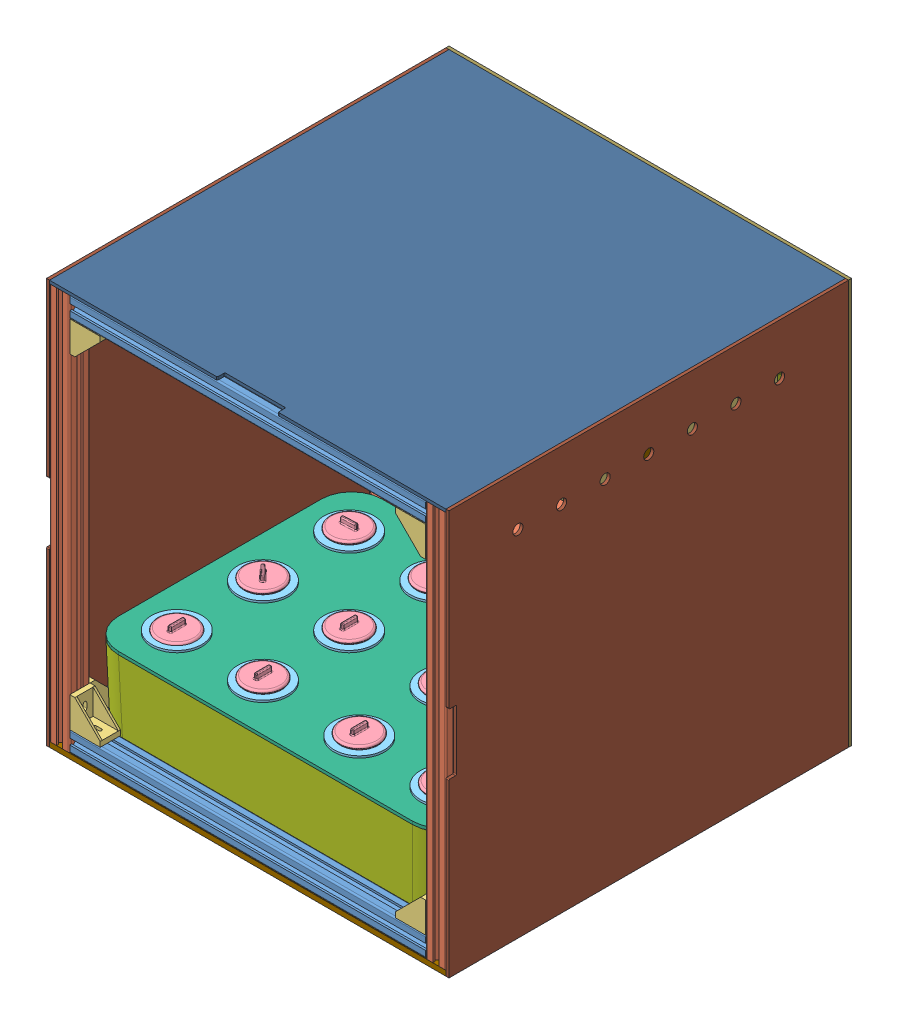
SolidWorks assembly skeleton_v2, configuration 預設. Lengths in mm. (continued)
Mates (geometry in assembly coordinates): (continued)
- 重合/共線/共點271: coincident aligned: plane of Fixedcomponent_middle-3 through (369.3054 -262.2141 340) normal (0 0 -1); plane of Fixedcomponent_middle-5 through (369.3054 -122.2141 340) normal (0 0 -1)
- 重合/共線/共點272: coincident aligned: plane of Fixedcomponent_middle-3 through (369.3054 -262.2141 340) normal (0 0 -1); plane of Fixedcomponent_middle-7 through (369.3054 -402.2141 340) normal (0 0 -1)
- 重合/共線/共點273: coincident aligned: plane of Fixedcomponent_middle-3 through (377.0554 -262.2141 340) normal (1 0 0); plane of Fixedcomponent_middle-7 through (377.0554 -402.2141 340) normal (1 0 0)
- 重合/共線/共點274: coincident anti-aligned: plane of Fixedcomponent_middle-3 through (341.8036 -262.2141 342.3593) normal (0 -1 0); plane of Fixedcomponent_middle-7 through (341.8036 -262.2141 342.3593) normal (0 1 0)
- 重合/共線/共點275: coincident anti-aligned: plane of Fixedcomponent_middle-9 through (21.3071 -262.2141 342.3593) normal (0 -1 0); plane of Fixedcomponent_middle-10 through (21.3071 -262.2141 342.3593) normal (0 1 0)
- 重合/共線/共點276: coincident aligned: plane of Fixedcomponent_middle-8 through (-13.9446 -402.2141 340) normal (-1 0 0); plane of Fixedcomponent_middle-9 through (-13.9446 -122.2141 340) normal (-1 0 0)
- 重合/共線/共點277: coincident aligned: plane of Fixedcomponent_middle-8 through (-13.9446 -402.2141 340) normal (-1 0 0); plane of Fixedcomponent_middle-10 through (-13.9446 -262.2141 340) normal (-1 0 0)
- 重合/共線/共點278: coincident aligned: plane of Fixedcomponent_middle-8 through (-6.1946 -402.2141 340) normal (0 0 -1); plane of Fixedcomponent_middle-10 through (-6.1946 -262.2141 340) normal (0 0 -1)
- 重合/共線/共點279: coincident aligned: plane of Fixedcomponent_middle-11 through (-13.9446 157.7859 340) normal (-1 0 0); plane of Fixedcomponent_middle-12 through (-13.9446 17.7859 340) normal (-1 0 0)
- 重合/共線/共點280: coincident aligned: plane of Fixedcomponent_middle-11 through (-6.1946 157.7859 340) normal (0 0 -1); plane of Fixedcomponent_middle-12 through (-6.1946 17.7859 340) normal (0 0 -1)
- 重合/共線/共點281: coincident anti-aligned: plane of Fixedcomponent_middle-9 through (21.3071 -122.2141 342.3593) normal (0 1 0); plane of Fixedcomponent_middle-12 through (21.3071 -122.2141 342.3593) normal (0 -1 0)
- 重合/共線/共點282: coincident aligned: plane of Fixedcomponent_middle-9 through (-6.1946 -122.2141 340) normal (0 0 -1); plane of Fixedcomponent_middle-12 through (-6.1946 17.7859 340) normal (0 0 -1)
- 重合/共線/共點283: coincident anti-aligned: plane of Fixedcomponent_middle-11 through (21.3071 17.7859 342.3593) normal (0 -1 0); plane of Fixedcomponent_middle-12 through (21.3071 17.7859 342.3593) normal (0 1 0)
- 重合/共線/共點284: coincident aligned: plane of Fixedcomponent_middle-9 through (-13.9446 -122.2141 344) normal (0 0 1); plane of Fixedcomponent_middle-10 through (-13.9446 -262.2141 344) normal (0 0 1)
- 重合/共線/共點285: coincident anti-aligned: plane of Fixedcomponent_middle-8 through (21.3071 -402.2141 342.3593) normal (0 1 0); plane of Fixedcomponent_middle-10 through (21.3071 -402.2141 342.3593) normal (0 -1 0)
- 重合/共線/共點286: coincident aligned: plane of Fixedcomponent_middle-10 through (-13.9446 -262.2141 340) normal (-1 0 0); plane of Fixedcomponent_middle-12 through (-13.9446 17.7859 340) normal (-1 0 0)
- 重合/共線/共點287: coincident aligned: plane of Fixedcomponent-13 through (-67.368 142.6997 267.7916) normal (0 0 1); plane of Fixedcomponent-14 through (-67.368 127.6997 267.7916) normal (0 0 1)
- 重合/共線/共點288: coincident anti-aligned: plane of Fixedcomponent-13 through (-32.1163 127.6997 266.1509) normal (0 -1 0); plane of Fixedcomponent-14 through (-32.1163 127.6997 266.1509) normal (0 1 0)
- 重合/共線/共點289: coincident aligned: plane of Fixedcomponent-14 through (-67.368 127.6997 263.7916) normal (-1 0 0); plane of Fixedcomponent-17 through (-67.368 112.6997 263.7916) normal (-1 0 0)
- 重合/共線/共點290: coincident anti-aligned: plane of Fixedcomponent-13 through (-32.1163 142.6997 266.1509) normal (0 1 0); plane of Fixedcomponent-16 through (-32.1163 142.6997 266.1509) normal (0 -1 0)
- 重合/共線/共點291: coincident aligned: plane of Fixedcomponent_middle-15 through (369.3054 -1242.2141 340) normal (0 0 -1); plane of Fixedcomponent-16 through (-59.618 157.6997 263.7916) normal (0 0 -1)
- 重合/共線/共點292: coincident aligned: plane of Fixedcomponent_middle-15 through (377.0554 -1242.2141 340) normal (1 0 0); plane of Fixedcomponent-16 through (-67.368 157.6997 263.7916) normal (-1 0 0)
- 重合/共線/共點293: coincident anti-aligned: plane of Fixedcomponent_middle-15 through (341.8036 -1102.2141 342.3593) normal (0 1 0); plane of Fixedcomponent-16 through (-32.1163 157.6997 266.1509) normal (0 1 0)
- 重合/共線/共點294: coincident aligned: plane of Fixedcomponent-13 through (-67.368 142.6997 263.7916) normal (-1 0 0); plane of Fixedcomponent-17 through (-67.368 112.6997 263.7916) normal (-1 0 0)
- 重合/共線/共點295: coincident anti-aligned: plane of Fixedcomponent-14 through (-32.1163 112.6997 266.1509) normal (0 -1 0); plane of Fixedcomponent-17 through (-32.1163 112.6997 266.1509) normal (0 1 0)
- 重合/共線/共點296: coincident aligned: plane of Fixedcomponent-13 through (-59.618 142.6997 263.7916) normal (0 0 -1); plane of Fixedcomponent-16 through (-59.618 157.6997 263.7916) normal (0 0 -1)
- 重合/共線/共點297: coincident aligned: plane of Fixedcomponent-14 through (-67.368 127.6997 263.7916) normal (-1 0 0); plane of Fixedcomponent-16 through (-67.368 157.6997 263.7916) normal (-1 0 0)
- 重合/共線/共點298: coincident aligned: plane of Fixedcomponent-14 through (-59.618 127.6997 263.7916) normal (0 0 -1); plane of Fixedcomponent-17 through (-59.618 112.6997 263.7916) normal (0 0 -1)
- 重合/共線/共點299: coincident aligned: plane of Fixedcomponent_middle-2 through (-13.9446 297.7859 340) normal (-1 0 0); plane of Fixedcomponent_middle-12 through (-13.9446 17.7859 340) normal (-1 0 0)
- 重合/共線/共點300: coincident anti-aligned: plane of Fixedcomponent_middle-2 through (21.3071 157.7859 342.3593) normal (0 -1 0); plane of Fixedcomponent_middle-11 through (21.3071 157.7859 342.3593) normal (0 1 0)
- 重合/共線/共點301: coincident aligned: plane of Fixedcomponent_middle-2 through (-6.1946 297.7859 340) normal (0 0 -1); plane of Fixedcomponent_middle-11 through (-6.1946 157.7859 340) normal (0 0 -1)
- 重合/共線/共點302: coincident aligned: plane of Fixedcomponent_middle-19 through (-13.9446 -542.2141 340) normal (-1 0 0); plane of Fixedcomponent_middle-20 through (-13.9446 -682.2141 340) normal (-1 0 0)
- 重合/共線/共點303: coincident aligned: plane of Fixedcomponent_middle-18 through (-13.9446 -962.2141 344) normal (0 0 1); plane of Fixedcomponent_middle-22 through (-13.9446 -822.2141 344) normal (0 0 1)
- 重合/共線/共點304: coincident anti-aligned: plane of Fixedcomponent_middle-18 through (21.3071 -962.2141 342.3593) normal (0 1 0); plane of Fixedcomponent_middle-22 through (21.3071 -962.2141 342.3593) normal (0 -1 0)
- 重合/共線/共點305: coincident aligned: plane of Fixedcomponent_middle-19 through (-6.1946 -542.2141 340) normal (0 0 -1); plane of Fixedcomponent_middle-20 through (-6.1946 -682.2141 340) normal (0 0 -1)
- 重合/共線/共點306: coincident anti-aligned: plane of Fixedcomponent_middle-20 through (21.3071 -822.2141 342.3593) normal (0 -1 0); plane of Fixedcomponent_middle-22 through (21.3071 -822.2141 342.3593) normal (0 1 0)
- 重合/共線/共點307: coincident anti-aligned: plane of Fixedcomponent_middle-19 through (21.3071 -682.2141 342.3593) normal (0 -1 0); plane of Fixedcomponent_middle-20 through (21.3071 -682.2141 342.3593) normal (0 1 0)
- 重合/共線/共點308: coincident aligned: plane of Fixedcomponent_middle-18 through (-13.9446 -962.2141 340) normal (-1 0 0); plane of Fixedcomponent_middle-21 through (-13.9446 -1102.2141 340) normal (-1 0 0)
- 重合/共線/共點309: coincident anti-aligned: plane of Fixedcomponent_middle-18 through (21.3071 -1102.2141 342.3593) normal (0 -1 0); plane of Fixedcomponent_middle-21 through (21.3071 -1102.2141 342.3593) normal (0 1 0)
- 重合/共線/共點310: coincident aligned: plane of Fixedcomponent_middle-18 through (-13.9446 -962.2141 340) normal (-1 0 0); plane of Fixedcomponent_middle-20 through (-13.9446 -682.2141 340) normal (-1 0 0)
- 重合/共線/共點311: coincident aligned: plane of Fixedcomponent_middle-18 through (-6.1946 -962.2141 340) normal (0 0 -1); plane of Fixedcomponent_middle-21 through (-6.1946 -1102.2141 340) normal (0 0 -1)
- 重合/共線/共點312: coincident aligned: plane of Fixedcomponent_middle-20 through (-6.1946 -682.2141 340) normal (0 0 -1); plane of Fixedcomponent_middle-22 through (-6.1946 -822.2141 340) normal (0 0 -1)
- 重合/共線/共點313: coincident aligned: plane of Fixedcomponent_middle-21 through (-13.9446 -1102.2141 340) normal (-1 0 0); plane of Fixedcomponent_middle-22 through (-13.9446 -822.2141 340) normal (-1 0 0)
- 重合/共線/共點314: coincident aligned: plane of Fixedcomponent_middle-24 through (297.0586 379.1322 340) normal (0 1 0); plane of Fixedcomponent_middle-25 through (157.0586 379.1322 340) normal (0 1 0)
- 重合/共線/共點315: coincident aligned: plane of Fixedcomponent_middle-23 through (-122.9414 379.1322 344) normal (0 0 1); plane of Fixedcomponent_middle-27 through (17.0586 379.1322 344) normal (0 0 1)
- 重合/共線/共點316: coincident anti-aligned: plane of Fixedcomponent_middle-23 through (-122.9414 343.8805 342.3593) normal (1 0 0); plane of Fixedcomponent_middle-27 through (-122.9414 343.8805 342.3593) normal (-1 0 0)
- 重合/共線/共點317: coincident aligned: plane of Fixedcomponent_middle-24 through (297.0586 371.3822 340) normal (0 0 -1); plane of Fixedcomponent_middle-25 through (157.0586 371.3822 340) normal (0 0 -1)
- 重合/共線/共點318: coincident anti-aligned: plane of Fixedcomponent_middle-25 through (17.0586 343.8805 342.3593) normal (-1 0 0); plane of Fixedcomponent_middle-27 through (17.0586 343.8805 342.3593) normal (1 0 0)
- 重合/共線/共點319: coincident anti-aligned: plane of Fixedcomponent_middle-24 through (157.0586 343.8805 342.3593) normal (-1 0 0); plane of Fixedcomponent_middle-25 through (157.0586 343.8805 342.3593) normal (1 0 0)
- 重合/共線/共點320: coincident aligned: plane of Fixedcomponent_middle-23 through (-122.9414 379.1322 340) normal (0 1 0); plane of Fixedcomponent_middle-26 through (-262.9414 379.1322 340) normal (0 1 0)
- 重合/共線/共點321: coincident anti-aligned: plane of Fixedcomponent_middle-23 through (-262.9414 343.8805 342.3593) normal (-1 0 0); plane of Fixedcomponent_middle-26 through (-262.9414 343.8805 342.3593) normal (1 0 0)
- 重合/共線/共點322: coincident aligned: plane of Fixedcomponent_middle-23 through (-122.9414 379.1322 340) normal (0 1 0); plane of Fixedcomponent_middle-25 through (157.0586 379.1322 340) normal (0 1 0)
- 重合/共線/共點323: coincident aligned: plane of Fixedcomponent_middle-23 through (-122.9414 371.3822 340) normal (0 0 -1); plane of Fixedcomponent_middle-26 through (-262.9414 371.3822 340) normal (0 0 -1)
- 重合/共線/共點324: coincident aligned: plane of Fixedcomponent_middle-25 through (157.0586 371.3822 340) normal (0 0 -1); plane of Fixedcomponent_middle-27 through (17.0586 371.3822 340) normal (0 0 -1)
- 重合/共線/共點325: coincident aligned: plane of Fixedcomponent_middle-26 through (-262.9414 379.1322 340) normal (0 1 0); plane of Fixedcomponent_middle-27 through (17.0586 379.1322 340) normal (0 1 0)
- 重合/共線/共點326: coincident aligned: plane of Fixedcomponent_middle-29 through (766.0522 379.1322 340) normal (0 1 0); plane of Fixedcomponent_middle-30 through (626.0522 379.1322 340) normal (0 1 0)
- 重合/共線/共點327: coincident aligned: plane of Fixedcomponent_middle-28 through (346.0522 379.1322 344) normal (0 0 1); plane of Fixedcomponent_middle-32 through (486.0522 379.1322 344) normal (0 0 1)
- 重合/共線/共點328: coincident anti-aligned: plane of Fixedcomponent_middle-28 through (346.0522 343.8805 342.3593) normal (1 0 0); plane of Fixedcomponent_middle-32 through (346.0522 343.8805 342.3593) normal (-1 0 0)
- 重合/共線/共點329: coincident aligned: plane of Fixedcomponent_middle-29 through (766.0522 371.3822 340) normal (0 0 -1); plane of Fixedcomponent_middle-30 through (626.0522 371.3822 340) normal (0 0 -1)
- 重合/共線/共點330: coincident anti-aligned: plane of Fixedcomponent_middle-30 through (486.0522 343.8805 342.3593) normal (-1 0 0); plane of Fixedcomponent_middle-32 through (486.0522 343.8805 342.3593) normal (1 0 0)
- 重合/共線/共點331: coincident anti-aligned: plane of Fixedcomponent_middle-29 through (626.0522 343.8805 342.3593) normal (-1 0 0); plane of Fixedcomponent_middle-30 through (626.0522 343.8805 342.3593) normal (1 0 0)
- 重合/共線/共點332: coincident aligned: plane of Fixedcomponent_middle-28 through (346.0522 379.1322 340) normal (0 1 0); plane of Fixedcomponent_middle-31 through (206.2372 379.1322 340) normal (0 1 0)
- 重合/共線/共點333: coincident anti-aligned: plane of Fixedcomponent_middle-28 through (206.0522 343.8805 342.3593) normal (-1 0 0); plane of Fixedcomponent_middle-31 through (206.2372 343.8805 342.3593) normal (1 0 0)
- 重合/共線/共點334: coincident aligned: plane of Fixedcomponent_middle-28 through (346.0522 379.1322 340) normal (0 1 0); plane of Fixedcomponent_middle-30 through (626.0522 379.1322 340) normal (0 1 0)
- 重合/共線/共點335: coincident aligned: plane of Fixedcomponent_middle-28 through (346.0522 371.3822 340) normal (0 0 -1); plane of Fixedcomponent_middle-31 through (206.2372 371.3822 340) normal (0 0 -1)
- 重合/共線/共點336: coincident aligned: plane of Fixedcomponent_middle-30 through (626.0522 371.3822 340) normal (0 0 -1); plane of Fixedcomponent_middle-32 through (486.0522 371.3822 340) normal (0 0 -1)
- 重合/共線/共點337: coincident aligned: plane of Fixedcomponent_middle-31 through (206.2372 379.1322 340) normal (0 1 0); plane of Fixedcomponent_middle-32 through (486.0522 379.1322 340) normal (0 1 0)
- 重合/共線/共點338: coincident aligned: plane of Fixedcomponent_middle-8 through (-13.9446 -402.2141 340) normal (-1 0 0); plane of Fixedcomponent_middle-19 through (-13.9446 -542.2141 340) normal (-1 0 0)
- 重合/共線/共點339: coincident aligned: plane of Fixedcomponent_middle-8 through (-6.1946 -402.2141 340) normal (0 0 -1); plane of Fixedcomponent_middle-20 through (-6.1946 -682.2141 340) normal (0 0 -1)
- 重合/共線/共點340: coincident anti-aligned: plane of Fixedcomponent_middle-8 through (21.3071 -542.2141 342.3593) normal (0 -1 0); plane of Fixedcomponent_middle-19 through (21.3071 -542.2141 342.3593) normal (0 1 0)
- 重合/共線/共點341: coincident anti-aligned: plane of Fixedcomponent_middle-34 through (1046.0522 343.8805 342.3593) normal (-1 0 0); plane of Fixedcomponent_middle-35 through (1046.0522 343.8805 342.3593) normal (1 0 0)
- 重合/共線/共點342: coincident aligned: plane of Fixedcomponent_middle-33 through (906.0522 379.1322 340) normal (0 1 0); plane of Fixedcomponent_middle-34 through (1186.0522 379.1322 340) normal (0 1 0)
- 重合/共線/共點343: coincident aligned: plane of Fixedcomponent_middle-33 through (906.0522 379.1322 340) normal (0 1 0); plane of Fixedcomponent_middle-35 through (1046.0522 379.1322 340) normal (0 1 0)
- 重合/共線/共點344: coincident aligned: plane of Fixedcomponent_middle-33 through (906.0522 371.3822 340) normal (0 0 -1); plane of Fixedcomponent_middle-35 through (1046.0522 371.3822 340) normal (0 0 -1)
- 重合/共線/共點345: coincident aligned: plane of Fixedcomponent_middle-36 through (1466.0522 379.1322 340) normal (0 1 0); plane of Fixedcomponent_middle-37 through (1326.0522 379.1322 340) normal (0 1 0)
- 重合/共線/共點346: coincident aligned: plane of Fixedcomponent_middle-36 through (1466.0522 371.3822 340) normal (0 0 -1); plane of Fixedcomponent_middle-37 through (1326.0522 371.3822 340) normal (0 0 -1)
- 重合/共線/共點347: coincident anti-aligned: plane of Fixedcomponent_middle-34 through (1186.0522 343.8805 342.3593) normal (1 0 0); plane of Fixedcomponent_middle-37 through (1186.0522 343.8805 342.3593) normal (-1 0 0)
- 重合/共線/共點348: coincident aligned: plane of Fixedcomponent_middle-34 through (1186.0522 371.3822 340) normal (0 0 -1); plane of Fixedcomponent_middle-37 through (1326.0522 371.3822 340) normal (0 0 -1)
- 重合/共線/共點349: coincident anti-aligned: plane of Fixedcomponent_middle-36 through (1326.0522 343.8805 342.3593) normal (-1 0 0); plane of Fixedcomponent_middle-37 through (1326.0522 343.8805 342.3593) normal (1 0 0)
- 重合/共線/共點350: coincident aligned: plane of Fixedcomponent_middle-34 through (1186.0522 379.1322 344) normal (0 0 1); plane of Fixedcomponent_middle-35 through (1046.0522 379.1322 344) normal (0 0 1)
- 重合/共線/共點351: coincident anti-aligned: plane of Fixedcomponent_middle-33 through (906.0522 343.8805 342.3593) normal (1 0 0); plane of Fixedcomponent_middle-35 through (906.0522 343.8805 342.3593) normal (-1 0 0)
- 重合/共線/共點352: coincident aligned: plane of Fixedcomponent_middle-35 through (1046.0522 379.1322 340) normal (0 1 0); plane of Fixedcomponent_middle-37 through (1326.0522 379.1322 340) normal (0 1 0)
- 重合/共線/共點353: coincident anti-aligned: plane of Fixedcomponent_middle-29 through (766.0522 343.8805 342.3593) normal (1 0 0); plane of Fixedcomponent_middle-33 through (766.0522 343.8805 342.3593) normal (-1 0 0)
- 重合/共線/共點354: coincident aligned: plane of Fixedcomponent_middle-30 through (626.0522 379.1322 340) normal (0 1 0); plane of Fixedcomponent_middle-33 through (906.0522 379.1322 340) normal (0 1 0)
- 重合/共線/共點355: coincident aligned: plane of Fixedcomponent_middle-29 through (766.0522 379.1322 344) normal (0 0 1); plane of Fixedcomponent_middle-33 through (906.0522 379.1322 344) normal (0 0 1)
- 重合/共線/共點357: coincident aligned: plane of FixedcomponentWithtri-2 through (66.2372 371.3822 340) normal (0 0 -1); plane of Fixedcomponent_middle-31 through (206.2372 371.3822 340) normal (0 0 -1)
- 重合/共線/共點358: coincident aligned: plane of FixedcomponentWithtri-2 through (66.2372 379.1322 340) normal (0 1 0); plane of Fixedcomponent_middle-31 through (206.2372 379.1322 340) normal (0 1 0)
- 重合/共線/共點359: coincident anti-aligned: plane of plate_side-2 through (377.0554 182.6322 514) normal (-1 0 0); plane of FixedcomponentWithtriright-1 through (377.0554 328.936 344) normal (1 0 0)
- 重合/共線/共點360: coincident anti-aligned: plane of plate_top-1 through (181.5554 379.1322 514) normal (0 -1 0); plane of FixedcomponentWithtriright-1 through (296.8586 379.1322 340) normal (0 1 0)
- 重合/共線/共點361: coincident anti-aligned: line of Fixedcomponent_middle-36 through (1466.0522 327.5188 320) axis (0 1 0); plane of FixedcomponentWithtriright-1 through (301.8586 343.8805 320) normal (0 0 -1)
- 重合/共線/共點362: coincident anti-aligned: plane of Fixedcomponent_middle-39 through (341.8036 -682.2141 342.3593) normal (0 1 0); plane of Fixedcomponent_middle-40 through (341.8036 -682.2141 342.3593) normal (0 -1 0)
- 重合/共線/共點363: coincident aligned: plane of Fixedcomponent_middle-38 through (377.0554 -542.2141 340) normal (1 0 0); plane of Fixedcomponent_middle-39 through (377.0554 -822.2141 340) normal (1 0 0)
- 重合/共線/共點364: coincident aligned: plane of Fixedcomponent_middle-38 through (377.0554 -542.2141 340) normal (1 0 0); plane of Fixedcomponent_middle-40 through (377.0554 -682.2141 340) normal (1 0 0)
- 重合/共線/共點365: coincident aligned: plane of Fixedcomponent_middle-38 through (369.3054 -542.2141 340) normal (0 0 -1); plane of Fixedcomponent_middle-40 through (369.3054 -682.2141 340) normal (0 0 -1)
- 重合/共線/共點366: coincident aligned: plane of Fixedcomponent_middle-41 through (377.0554 -1102.2141 340) normal (1 0 0); plane of Fixedcomponent_middle-42 through (377.0554 -962.2141 340) normal (1 0 0)
- 重合/共線/共點367: coincident aligned: plane of Fixedcomponent_middle-41 through (369.3054 -1102.2141 340) normal (0 0 -1); plane of Fixedcomponent_middle-42 through (369.3054 -962.2141 340) normal (0 0 -1)
- 重合/共線/共點368: coincident anti-aligned: plane of Fixedcomponent_middle-39 through (341.8036 -822.2141 342.3593) normal (0 -1 0); plane of Fixedcomponent_middle-42 through (341.8036 -822.2141 342.3593) normal (0 1 0)
- 重合/共線/共點369: coincident aligned: plane of Fixedcomponent_middle-39 through (369.3054 -822.2141 340) normal (0 0 -1); plane of Fixedcomponent_middle-42 through (369.3054 -962.2141 340) normal (0 0 -1)
- 重合/共線/共點370: coincident anti-aligned: plane of Fixedcomponent_middle-41 through (341.8036 -962.2141 342.3593) normal (0 1 0); plane of Fixedcomponent_middle-42 through (341.8036 -962.2141 342.3593) normal (0 -1 0)
- 重合/共線/共點371: coincident aligned: plane of Fixedcomponent_middle-39 through (377.0554 -822.2141 344) normal (0 0 1); plane of Fixedcomponent_middle-40 through (377.0554 -682.2141 344) normal (0 0 1)
- 重合/共線/共點372: coincident anti-aligned: plane of Fixedcomponent_middle-38 through (341.8036 -542.2141 342.3593) normal (0 -1 0); plane of Fixedcomponent_middle-40 through (341.8036 -542.2141 342.3593) normal (0 1 0)
- 重合/共線/共點373: coincident aligned: plane of Fixedcomponent_middle-40 through (377.0554 -682.2141 340) normal (1 0 0); plane of Fixedcomponent_middle-42 through (377.0554 -962.2141 340) normal (1 0 0)
- 重合/共線/共點386: coincident anti-aligned: plane of Fixedcomponent_middle-7 through (341.8036 -402.2141 342.3593) normal (0 -1 0); plane of Fixedcomponent_middle-38 through (341.8036 -402.2141 342.3593) normal (0 1 0)
- 重合/共線/共點387: coincident aligned: plane of Fixedcomponent_middle-7 through (377.0554 -402.2141 344) normal (0 0 1); plane of Fixedcomponent_middle-38 through (377.0554 -542.2141 344) normal (0 0 1)
- 重合/共線/共點388: coincident aligned: plane of Fixedcomponent_middle-7 through (377.0554 -402.2141 340) normal (1 0 0); plane of Fixedcomponent_middle-38 through (377.0554 -542.2141 340) normal (1 0 0)
- 重合/共線/共點389: coincident anti-aligned: plane of Fixedcomponent_middle-24 through (297.0586 343.8805 342.3593) normal (1 0 0); plane of FixedcomponentWithtriright-1 through (296.8586 343.8805 342.3593) normal (-1 0 0)
- 重合/共線/共點390: coincident anti-aligned: plane of plate_back-1 through (181.5554 183.6322 320) normal (0 0 1); plane of Fixedcomponent_middle-26 through (-262.9414 331.3488 320) normal (0 0 -1)
- 重合/共線/共點391: coincident aligned: plane of Fixedcomponent_middle-26 through (-262.9414 379.1322 340) normal (0 1 0); plane of Fixedcomponent_middle-36 through (1466.0522 379.1322 340) normal (0 1 0)
- 重合/共線/共點392: coincident anti-aligned: plane of plate_side-2 through (377.0554 182.6322 514) normal (-1 0 0); plane of Fixedcomponent_middle-41 through (377.0554 -1102.2141 340) normal (1 0 0)
- 重合/共線/共點393: coincident anti-aligned: plane of plate_back-1 through (181.5554 183.6322 320) normal (0 0 1); plane of Fixedcomponent_middle-42 through (329.272 -962.2141 320) normal (0 0 -1)
- 重合/共線/共點394: coincident anti-aligned: plane of Fixedcomponent-4 through (341.8036 297.7859 342.3593) normal (0 1 0); plane of FixedcomponentWithtriright-1 through (353.1054 297.7859 320) normal (0 -1 0)
- 重合/共線/共點395: coincident anti-aligned: plane of plate_side-2 through (377.0554 182.6322 514) normal (-1 0 0); plane of Fixedcomponent_middle-15 through (377.0554 -1242.2141 340) normal (1 0 0)
- 重合/共線/共點396: coincident anti-aligned: plane of plate_back-1 through (181.5554 183.6322 320) normal (0 0 1); plane of Fixedcomponent_middle-15 through (329.272 -1242.2141 320) normal (0 0 -1)
- 重合/共線/共點397: coincident anti-aligned: plane of Fixedcomponent_middle-15 through (341.8036 -1102.2141 342.3593) normal (0 1 0); plane of Fixedcomponent_middle-41 through (341.8036 -1102.2141 342.3593) normal (0 -1 0)
- 重合/共線/共點398: coincident aligned: plane of Fixedcomponent_middle-15 through (341.8036 -1242.2141 342.3593) normal (0 -1 0); plane of Assem1-1/raspberry pi test-1 through (206.2372 144.5864 322) normal (0 -1 0)
- 重合/共線/共點400: coincident: line of Fixedcomponent_middle-37 through (1326.0522 379.1322 344) axis (0 -1 0); plane of Assem1-1/raspberry pi test-1 through (206.2372 144.5864 322) normal (1 0 0)
- 重合/共線/共點401: coincident anti-aligned: plane of plate_back-1 through (181.5554 183.6322 320) normal (0 0 1); plane of Assem1-1/raspberry pi test-1 through (185.8137 159.8307 320) normal (0 0 -1)
- 重合/共線/共點402: coincident: line of plate_side-2 through (380.0554 -16.8678 317) axis (0 1 0); plane of plate_door-2 through (181.5554 182.6322 317) normal (0 0 1)
- 重合/共線/共點403: coincident anti-aligned: plane of controlbox_right-3 through (106.0554 78.1322 433) normal (-1 0 0); plane of controlbox_left-1 through (106.0554 63.1322 340) normal (1 0 0)
- 重合/共線/共點404: coincident anti-aligned: plane of plate_bottom-1 through (181.5554 -11.8678 514) normal (0 1 0); plane of 1219 ControlBox version-1/1219 ground-1 through (357.0554 -11.8678 419) normal (0 -1 0)
- 重合/共線/共點410: coincident anti-aligned: plane of stick_2020_340-8 through (357.0554 8.1322 340) normal (0 0 1); plane of 1219 ControlBox version-1/1219 roof-1 through (320.6845 26.144 340) normal (0 0 -1)
- 重合/共線/共點413: coincident anti-aligned: plane of stick_2020_340-6 through (357.0554 8.1322 340) normal (-1 0 0); plane of 1219 ControlBox version-1/1219 ground-1 through (357.0554 76.1322 419) normal (1 0 0)
- 重合/共線/共點415: coincident anti-aligned: plane of stick_2020_340-1 through (6.0554 8.1322 691) normal (1 0 0); plane of controlbox_left-1 through (6.0554 71.1322 433) normal (-1 0 0)
- 重合/共線/共點416: coincident anti-aligned: plane of stick_2020_340-8 through (357.0554 8.1322 340) normal (0 0 1); plane of controlbox_left-1 through (116.0554 71.1322 340) normal (0 0 -1)
- 重合/共線/共點417: coincident anti-aligned: plane of controlbox_left-1 through (116.0554 71.1322 386.5) normal (0 1 0); plane of controlbox_lid-1 through (116.1055 71.1322 386.7449) normal (0 -1 0)
- 相切2: tangent aligned: cylinder of controlbox_lid-1 through (196.1556 66.1322 370.4898) axis (0 1 0) radius 25.5; cylinder of controlbox_left-1 through (196.0554 71.1322 370) axis (0 -1 0) radius 26
- 同軸心20: concentric aligned: cylinder of controlbox_left-1 through (36.0554 71.1322 403) axis (0 1 0) radius 26; cylinder of controlbox_lid-1 through (36.0554 66.1322 403) axis (0 1 0) radius 25.5
- 重合/共線/共點418: coincident anti-aligned: plane of lid_v2-1 through (181.0554 81.1322 562.9859) normal (0 1 0); plane of ring-15 through (228.5554 81.1322 477.9859) normal (0 -1 0)
- 重合/共線/共點419: coincident anti-aligned: plane of lid_v2-1 through (181.0554 81.1322 562.9859) normal (0 1 0); plane of ring-11 through (313.5554 81.1322 477.9859) normal (0 -1 0)
- 重合/共線/共點420: coincident anti-aligned: plane of lid_v2-1 through (181.0554 81.1322 562.9859) normal (0 1 0); plane of ring-14 through (228.5554 81.1322 562.9859) normal (0 -1 0)
- 重合/共線/共點421: coincident anti-aligned: plane of lid_v2-1 through (181.0554 81.1322 562.9859) normal (0 1 0); plane of ring-13 through (228.5554 81.1322 647.9859) normal (0 -1 0)
- 重合/共線/共點422: coincident anti-aligned: plane of lid_v2-1 through (181.0554 81.1322 562.9859) normal (0 1 0); plane of ring-12 through (313.5554 81.1322 562.9859) normal (0 -1 0)
- 同軸心21: concentric aligned: cylinder of lid_v2-1 through (228.5554 78.1312 477.9859) axis (0 1 0) radius 22; cylinder of ring-15 through (228.5554 77.8822 477.9859) axis (0 1 0) radius 15.5
- 同軸心22: concentric aligned: cylinder of lid_v2-1 through (228.5554 78.1312 562.9859) axis (0 1 0) radius 22; cylinder of ring-14 through (228.5554 77.8822 562.9859) axis (0 1 0) radius 15.5
- 同軸心23: concentric aligned: cylinder of lid_v2-1 through (228.5554 78.1312 647.9859) axis (0 1 0) radius 22; cylinder of ring-13 through (228.5554 77.8822 647.9859) axis (0 1 0) radius 15.5
- 同軸心24: concentric aligned: cylinder of lid_v2-1 through (313.5554 78.1312 477.9859) axis (0 1 0) radius 22; cylinder of ring-11 through (313.5554 77.8822 477.9859) axis (0 1 0) radius 15.5
- 同軸心25: concentric aligned: cylinder of lid_v2-1 through (313.5554 78.1312 562.9859) axis (0 1 0) radius 22; cylinder of ring-12 through (313.5554 77.8822 562.9859) axis (0 1 0) radius 15.5
- 重合/共線/共點423: coincident anti-aligned: plane of lid_v2-1 through (181.0554 81.1322 562.9859) normal (0 1 0); plane of ring-16 through (313.5554 81.1322 647.9859) normal (0 -1 0)
- 同軸心26: concentric aligned: cylinder of lid_v2-1 through (313.5554 78.1312 647.9859) axis (0 1 0) radius 22; cylinder of ring-16 through (313.5554 77.8822 647.9859) axis (0 1 0) radius 15.5
- 同軸心27: concentric aligned: cylinder of ring-1 through (48.5554 77.8822 477.9859) axis (0 1 0) radius 15.5; cylinder of small fixed lid with EC sensor and temperture-1 through (48.5554 79.1322 477.9859) axis (0 1 0) radius 14.75
- 重合/共線/共點424: coincident anti-aligned: plane of ring-1 through (48.5554 83.1322 477.9859) normal (0 1 0); plane of small fixed lid with EC sensor and temperture-4 through (19.7064 83.1322 641.3464) normal (0 -1 0)
- 重合/共線/共點425: coincident anti-aligned: plane of ring-9 through (133.5554 83.1322 562.9859) normal (0 1 0); plane of small fixed lid with EC sensor and temperture-2 through (104.7064 83.1322 556.3464) normal (0 -1 0)
- 重合/共線/共點426: coincident anti-aligned: plane of ring-3 through (48.5554 83.1322 647.9859) normal (0 1 0); plane of small fixed lid with EC sensor and temperture-1 through (25.7411 83.1322 496.85) normal (0 -1 0)
- 重合/共線/共點427: coincident anti-aligned: plane of ring-14 through (228.5554 83.1322 562.9859) normal (0 1 0); plane of small fixed lid with EC sensor and temperture-5 through (199.7064 83.1322 556.3464) normal (0 -1 0)
- 重合/共線/共點428: coincident anti-aligned: plane of ring-11 through (313.5554 83.1322 477.9859) normal (0 1 0); plane of small fixed lid with EC sensor and temperture-3 through (329.9868 83.1034 508.6938) normal (0 -1 0)
- 重合/共線/共點429: coincident anti-aligned: plane of ring-16 through (313.5554 83.1322 647.9859) normal (0 1 0); plane of small fixed lid with EC sensor and temperture-6 through (284.7064 83.1322 556.3464) normal (0 -1 0)
- 同軸心28: concentric aligned: cylinder of ring-3 through (48.5554 77.8822 647.9859) axis (0 1 0) radius 15.5; cylinder of small fixed lid with EC sensor and temperture-4 through (48.5554 79.1322 647.9859) axis (0 1 0) radius 14.75
- 同軸心29: concentric aligned: cylinder of ring-9 through (133.5554 77.8822 562.9859) axis (0 1 0) radius 15.5; cylinder of small fixed lid with EC sensor and temperture-2 through (133.5554 79.1322 562.9859) axis (0 1 0) radius 14.75
- 同軸心30: concentric aligned: cylinder of ring-14 through (228.5554 77.8822 562.9859) axis (0 1 0) radius 15.5; cylinder of small fixed lid with EC sensor and temperture-5 through (228.5554 79.1322 562.9859) axis (0 1 0) radius 14.75
- 重合/共線/共點430: coincident anti-aligned: plane of plate_back-1 through (181.5554 183.6322 320) normal (0 0 1); plane of Assem1-1/raspberry pi test-1 through (185.8137 159.8307 320) normal (0 0 -1)
- 重合/共線/共點431: coincident aligned: plane of Fixedcomponent_middle-2 through (21.3071 157.7859 342.3593) normal (0 -1 0); plane of Assem1-1/raspberry pi test-1 through (206.2372 144.5864 322) normal (0 -1 0)
- 重合/共線/共點432: coincident anti-aligned: plane of FixedcomponentWithtri-2 through (10.0054 297.7683 320) normal (0 -1 0); plane of Fixedcomponent_left-43 through (21.3071 297.7683 342.3593) normal (0 1 0)
- 重合/共線/共點433: coincident aligned: plane of FixedcomponentWithtri-2 through (61.2372 343.8805 340) normal (0 0 -1); plane of Fixedcomponent_left-43 through (-6.1946 297.7683 340) normal (0 0 -1)
- 重合/共線/共點434: coincident aligned: plane of FixedcomponentWithtri-2 through (-13.9446 328.921 344) normal (-1 0 0); plane of Fixedcomponent_left-43 through (-13.9446 297.7683 340) normal (-1 0 0)
- 重合/共線/共點435: coincident aligned: plane of FixedcomponentWithtriright-1 through (377.0554 328.936 344) normal (1 0 0); plane of Fixedcomponent_right-43 through (377.0554 97.7859 340) normal (1 0 0)
- 重合/共線/共點436: coincident anti-aligned: plane of FixedcomponentWithtriright-1 through (353.1054 297.7859 320) normal (0 -1 0); plane of Fixedcomponent_right-43 through (341.8036 297.7859 342.3593) normal (0 1 0)
- 重合/共線/共點438: coincident anti-aligned: plane of plate_back-1 through (181.5554 183.6322 320) normal (0 0 1); plane of Fixedcomponent_right-43 through (329.472 97.7859 320) normal (0 0 -1)
- 重合/共線/共點439: coincident aligned: plane of Fixedcomponent_middle-31 through (206.2372 343.8805 342.3593) normal (1 0 0); plane of Assem1-1/raspberry pi test-1 through (206.2372 144.5864 322) normal (1 0 0)
- 重合/共線/共點440: coincident anti-aligned: plane of Fixedcomponent_right-43 through (341.8036 297.7859 342.3593) normal (0 1 0); plane of FixedcomponentWithtriright-2 through (353.1054 297.7859 320) normal (0 -1 0)
- 重合/共線/共點441: coincident aligned: plane of Fixedcomponent_right-43 through (377.0554 97.7859 340) normal (1 0 0); plane of FixedcomponentWithtriright-2 through (377.0554 328.9386 344) normal (1 0 0)
- 重合/共線/共點442: coincident anti-aligned: plane of stick_2020_380-4 through (357.0554 -11.8678 340) normal (0 0 1); plane of FixedcomponentWithtriright-2 through (301.8736 343.8981 340) normal (0 0 -1)
- 重合/共線/共點444: coincident aligned: plane of stick_2020_380-4 through (377.0554 -11.8678 320) normal (1 0 0); plane of FixedcomponentWithtriright-2 through (377.0554 328.9386 344) normal (1 0 0)
- 重合/共線/共點445: coincident anti-aligned: plane of FixedcomponentWithtri-2 through (66.2372 343.8805 342.3593) normal (1 0 0); plane of Fixedcomponent_middle-31 through (66.2372 343.8805 342.3593) normal (-1 0 0)
- 重合/共線/共點446: coincident: plane of stick_2020_380-2 through (-13.9446 -11.8678 340) normal (0 0 1); plane of 90 Degree Cast Corner for 2020 Extrusion (Ooznest).step-1 through (-5.4446 349.1322 340) normal (0 0 -1)
- 重合/共線/共點447: coincident: plane of stick_2020_340-3 through (-13.9446 359.1322 691) normal (0 -1 0); plane of 90 Degree Cast Corner for 2020 Extrusion (Ooznest).step-1 through (3.0554 359.1322 340) normal (0 1 0)
- 重合/共線/共點448: coincident aligned: plane of stick_2020_380-2 through (-13.9446 -11.8678 320) normal (-1 0 0); plane of 90 Degree Cast Corner for 2020 Extrusion (Ooznest).step-1 through (-13.9446 359.1322 340) normal (-1 0 0)
- 重合/共線/共點449: coincident anti-aligned: plane of stick_2020_380-2 through (-13.9446 -11.8678 340) normal (0 0 1); plane of Aluminium extrusion connector-1 through (6.0554 359.1322 340) normal (0 0 -1)
- 重合/共線/共點450: coincident anti-aligned: plane of stick_2020_340-3 through (-13.9446 359.1322 691) normal (0 -1 0); plane of Aluminium extrusion connector-1 through (6.0554 359.1322 370) normal (0 1 0)
- 重合/共線/共點451: coincident aligned: plane of stick_2020_340-3 through (-13.9446 379.1322 691) normal (-1 0 0); plane of Aluminium extrusion connector-1 through (-13.9446 359.1322 370) normal (-1 0 0)
- 重合/共線/共點452: coincident anti-aligned: plane of stick_2020_380-4 through (357.0554 -11.8678 340) normal (0 0 1); plane of Aluminium extrusion connector-5 through (377.0554 359.1322 340) normal (0 0 -1)
- 重合/共線/共點453: coincident anti-aligned: plane of stick_2020_340-7 through (377.0554 359.1322 340) normal (0 -1 0); plane of Aluminium extrusion connector-5 through (377.0554 359.1322 370) normal (0 1 0)
- 重合/共線/共點454: coincident aligned: plane of stick_2020_380-4 through (377.0554 -11.8678 320) normal (1 0 0); plane of Aluminium extrusion connector-5 through (377.0554 359.1322 370) normal (1 0 0)
- 重合/共線/共點455: coincident anti-aligned: plane of stick_2020_340-7 through (377.0554 359.1322 340) normal (0 -1 0); plane of Aluminium extrusion connector-4 through (357.0554 359.1322 661) normal (0 1 0)
- 重合/共線/共點456: coincident anti-aligned: plane of stick_2020_380-3 through (357.0554 -11.8678 691) normal (0 0 -1); plane of Aluminium extrusion connector-4 through (357.0554 359.1322 691) normal (0 0 1)
- 重合/共線/共點457: coincident aligned: plane of stick_2020_340-7 through (377.0554 379.1322 340) normal (1 0 0); plane of Aluminium extrusion connector-4 through (377.0554 359.1322 661) normal (1 0 0)
- 重合/共線/共點458: coincident anti-aligned: plane of stick_2020_340-4 through (6.0554 359.1322 691) normal (0 -1 0); plane of Aluminium extrusion connector-2 through (357.0554 359.1322 691) normal (0 1 0)
- 重合/共線/共點459: coincident anti-aligned: plane of stick_2020_380-3 through (357.0554 -11.8678 691) normal (-1 0 0); plane of Aluminium extrusion connector-2 through (357.0554 329.1322 691) normal (1 0 0)
- 重合/共線/共點460: coincident aligned: plane of stick_2020_340-4 through (6.0554 379.1322 711) normal (0 0 1); plane of Aluminium extrusion connector-2 through (357.0554 329.1322 711) normal (0 0 1)
- 重合/共線/共點461: coincident anti-aligned: plane of stick_2020_340-4 through (6.0554 379.1322 691) normal (0 0 -1); plane of Aluminium extrusion connector-3 through (327.0554 359.1322 691) normal (0 0 1)
- 重合/共線/共點462: coincident anti-aligned: plane of stick_2020_340-7 through (357.0554 379.1322 340) normal (-1 0 0); plane of Aluminium extrusion connector-3 through (357.0554 359.1322 691) normal (1 0 0)
- 重合/共線/共點463: coincident aligned: plane of stick_2020_340-7 through (377.0554 359.1322 340) normal (0 -1 0); plane of Aluminium extrusion connector-3 through (327.0554 359.1322 691) normal (0 -1 0)
- 重合/共線/共點464: coincident anti-aligned: plane of stick_2020_380-4 through (357.0554 -11.8678 320) normal (-1 0 0); plane of Aluminium extrusion connector-9 through (357.0554 359.1322 340) normal (1 0 0)
- 重合/共線/共點465: coincident anti-aligned: plane of stick_2020_340-5 through (6.0554 359.1322 320) normal (0 -1 0); plane of Aluminium extrusion connector-9 through (327.0554 359.1322 340) normal (0 1 0)
- 重合/共線/共點466: coincident aligned: plane of stick_2020_380-4 through (357.0554 -11.8678 320) normal (0 0 -1); plane of Aluminium extrusion connector-9 through (327.0554 359.1322 320) normal (0 0 -1)
- 重合/共線/共點467: coincident anti-aligned: plane of stick_2020_380-4 through (357.0554 -11.8678 340) normal (0 0 1); plane of Aluminium extrusion connector-7 through (357.0554 8.1322 340) normal (0 0 -1)
- 重合/共線/共點468: coincident anti-aligned: plane of stick_2020_340-6 through (377.0554 8.1322 340) normal (0 1 0); plane of Aluminium extrusion connector-7 through (357.0554 8.1322 370) normal (0 -1 0)
- 重合/共線/共點469: coincident aligned: plane of stick_2020_380-4 through (377.0554 -11.8678 320) normal (1 0 0); plane of Aluminium extrusion connector-7 through (377.0554 8.1322 370) normal (1 0 0)
- 重合/共線/共點470: coincident anti-aligned: plane of stick_2020_340-4 through (6.0554 379.1322 691) normal (0 0 -1); plane of Aluminium extrusion connector-8 through (6.0554 359.1322 691) normal (0 0 1)
- 重合/共線/共點471: coincident anti-aligned: plane of stick_2020_340-3 through (6.0554 379.1322 691) normal (1 0 0); plane of Aluminium extrusion connector-8 through (6.0554 359.1322 661) normal (-1 0 0)
- 重合/共線/共點472: coincident aligned: plane of stick_2020_340-3 through (-13.9446 379.1322 691) normal (0 1 0); plane of Aluminium extrusion connector-8 through (6.0554 379.1322 661) normal (0 1 0)
- 重合/共線/共點473: coincident anti-aligned: plane of Aluminium extrusion connector-6 through (6.0554 329.1322 691) normal (0 0 1); plane of stick_2020_380-1 through (-13.9446 -11.8678 691) normal (0 0 -1)
- 重合/共線/共點474: coincident anti-aligned: plane of stick_2020_340-3 through (-13.9446 359.1322 691) normal (0 -1 0); plane of Aluminium extrusion connector-6 through (6.0554 359.1322 691) normal (0 1 0)
- 重合/共線/共點476: coincident aligned: plane of stick_2020_340-3 through (-13.9446 379.1322 691) normal (-1 0 0); plane of Aluminium extrusion connector-6 through (-13.9446 329.1322 691) normal (-1 0 0)
- 重合/共線/共點477: coincident aligned: plane of stick_2020_380-1 through (-13.9446 -11.8678 711) normal (0 0 1); plane of Aluminium extrusion connector-18 through (6.0554 38.1322 711) normal (0 0 1)
- 重合/共線/共點478: coincident anti-aligned: plane of stick_2020_340-2 through (6.0554 8.1322 691) normal (0 1 0); plane of Aluminium extrusion connector-18 through (6.0554 8.1322 691) normal (0 -1 0)
- 重合/共線/共點479: coincident anti-aligned: plane of stick_2020_380-1 through (6.0554 -11.8678 691) normal (1 0 0); plane of Aluminium extrusion connector-18 through (6.0554 38.1322 691) normal (-1 0 0)
- 重合/共線/共點480: coincident anti-aligned: plane of stick_2020_340-1 through (-13.9446 8.1322 691) normal (0 1 0); plane of Aluminium extrusion connector-19 through (-13.9446 8.1322 691) normal (0 -1 0)
- 重合/共線/共點481: coincident anti-aligned: plane of stick_2020_380-1 through (-13.9446 -11.8678 691) normal (0 0 -1); plane of Aluminium extrusion connector-19 through (-13.9446 38.1322 691) normal (0 0 1)
- 重合/共線/共點482: coincident aligned: plane of stick_2020_380-1 through (-13.9446 -11.8678 691) normal (-1 0 0); plane of Aluminium extrusion connector-19 through (-13.9446 38.1322 691) normal (-1 0 0)
- 重合/共線/共點483: coincident anti-aligned: plane of stick_2020_380-2 through (6.0554 -11.8678 320) normal (1 0 0); plane of Aluminium extrusion connector-17 through (6.0554 38.1322 320) normal (-1 0 0)
- 重合/共線/共點484: coincident aligned: plane of stick_2020_380-2 through (-13.9446 -11.8678 340) normal (0 0 1); plane of Aluminium extrusion connector-17 through (6.0554 38.1322 340) normal (0 0 1)
- 重合/共線/共點485: coincident anti-aligned: plane of stick_2020_340-8 through (357.0554 8.1322 320) normal (0 1 0); plane of Aluminium extrusion connector-17 through (6.0554 8.1322 320) normal (0 -1 0)
- 重合/共線/共點486: coincident anti-aligned: plane of stick_2020_380-4 through (357.0554 -11.8678 320) normal (-1 0 0); plane of Aluminium extrusion connector-16 through (357.0554 38.1322 340) normal (1 0 0)
- 重合/共線/共點487: coincident anti-aligned: plane of stick_2020_340-8 through (357.0554 8.1322 320) normal (0 1 0); plane of Aluminium extrusion connector-16 through (357.0554 8.1322 340) normal (0 -1 0)
- 重合/共線/共點488: coincident aligned: plane of stick_2020_380-4 through (357.0554 -11.8678 320) normal (0 0 -1); plane of Aluminium extrusion connector-16 through (357.0554 38.1322 320) normal (0 0 -1)
- 重合/共線/共點489: coincident anti-aligned: plane of stick_2020_380-2 through (-13.9446 -11.8678 340) normal (0 0 1); plane of Aluminium extrusion connector-13 through (6.0554 38.1322 340) normal (0 0 -1)
- 重合/共線/共點490: coincident anti-aligned: plane of stick_2020_340-1 through (-13.9446 8.1322 691) normal (0 1 0); plane of Aluminium extrusion connector-13 through (6.0554 8.1322 340) normal (0 -1 0)
- 重合/共線/共點491: coincident aligned: plane of stick_2020_380-2 through (-13.9446 -11.8678 320) normal (-1 0 0); plane of Aluminium extrusion connector-13 through (-13.9446 38.1322 340) normal (-1 0 0)
- 重合/共線/共點493: coincident anti-aligned: plane of stick_2020_340-5 through (6.0554 359.1322 320) normal (0 -1 0); plane of Aluminium extrusion connector-15 through (6.0554 359.1322 340) normal (0 1 0)
- 重合/共線/共點494: coincident aligned: plane of stick_2020_340-5 through (6.0554 379.1322 320) normal (0 0 -1); plane of Aluminium extrusion connector-15 through (6.0554 329.1322 320) normal (0 0 -1)
- 重合/共線/共點495: coincident anti-aligned: plane of stick_2020_380-2 through (6.0554 -11.8678 320) normal (1 0 0); plane of Aluminium extrusion connector-15 through (6.0554 329.1322 340) normal (-1 0 0)
- 重合/共線/共點496: coincident anti-aligned: plane of stick_2020_380-1 through (6.0554 -11.8678 691) normal (1 0 0); plane of Aluminium extrusion connector-20 through (6.0554 359.1322 691) normal (-1 0 0)
- 重合/共線/共點497: coincident anti-aligned: plane of stick_2020_340-4 through (6.0554 359.1322 691) normal (0 -1 0); plane of Aluminium extrusion connector-20 through (36.0554 359.1322 691) normal (0 1 0)
- 重合/共線/共點498: coincident aligned: plane of stick_2020_380-1 through (-13.9446 -11.8678 711) normal (0 0 1); plane of Aluminium extrusion connector-20 through (36.0554 359.1322 711) normal (0 0 1)
- 重合/共線/共點499: coincident anti-aligned: plane of stick_2020_340-6 through (377.0554 8.1322 340) normal (0 1 0); plane of Aluminium extrusion connector-14 through (357.0554 8.1322 691) normal (0 -1 0)
- 重合/共線/共點500: coincident anti-aligned: plane of stick_2020_380-3 through (357.0554 -11.8678 691) normal (0 0 -1); plane of Aluminium extrusion connector-14 through (357.0554 38.1322 691) normal (0 0 1)
- 重合/共線/共點501: coincident aligned: plane of stick_2020_380-3 through (377.0554 -11.8678 691) normal (1 0 0); plane of Aluminium extrusion connector-14 through (377.0554 38.1322 691) normal (1 0 0)
- 重合/共線/共點502: coincident anti-aligned: plane of stick_2020_340-2 through (6.0554 8.1322 691) normal (0 1 0); plane of Aluminium extrusion connector-12 through (357.0554 8.1322 711) normal (0 -1 0)
- 重合/共線/共點503: coincident anti-aligned: plane of stick_2020_380-3 through (357.0554 -11.8678 691) normal (-1 0 0); plane of Aluminium extrusion connector-12 through (357.0554 38.1322 711) normal (1 0 0)
- 重合/共線/共點504: coincident aligned: plane of stick_2020_380-3 through (357.0554 -11.8678 711) normal (0 0 1); plane of Aluminium extrusion connector-12 through (357.0554 38.1322 711) normal (0 0 1)
- 重合/共線/共點505: coincident anti-aligned: plane of lid_v2-1 through (181.0554 81.1322 562.9859) normal (0 1 0); plane of ring-17 through (48.5554 81.1322 477.9859) normal (0 -1 0)
- 同軸心33: concentric aligned: cylinder of lid_v2-1 through (48.5554 78.1312 477.9859) axis (0 1 0) radius 22; cylinder of ring-17 through (48.5554 77.8822 477.9859) axis (0 1 0) radius 15.5
- 同軸心34: concentric aligned: cylinder of ring-2 through (48.5554 77.8822 562.9859) axis (0 1 0) radius 15.5; cylinder of small lid-1 through (48.5554 73.1322 562.9859) axis (0 1 0) radius 14.5
- 重合/共線/共點506: coincident anti-aligned: plane of ring-2 through (48.5554 83.1322 562.9859) normal (0 1 0); plane of small lid-1 through (48.5554 83.1322 562.9859) normal (0 -1 0)
- 同軸心35: concentric aligned: cylinder of small fixed lid with EC sensor and temperture-6 through (313.5554 79.1322 562.9859) axis (0 1 0) radius 14.75; cylinder of ring-12 through (313.5554 77.8822 562.9859) axis (0 1 0) radius 15.5
- 重合/共線/共點507: coincident anti-aligned: plane of lid_v2-1 through (181.0554 81.1322 562.9859) normal (0 1 0); plane of small lid-2 through (48.5554 81.1322 647.9859) normal (0 -1 0)
- 同軸心36: concentric aligned: cylinder of ring-3 through (48.5554 77.8822 647.9859) axis (0 1 0) radius 15.5; cylinder of small lid-2 through (48.5554 71.1322 647.9859) axis (0 1 0) radius 14.5
- 重合/共線/共點508: coincident anti-aligned: plane of ring-10 through (133.5554 83.1322 647.9859) normal (0 1 0); plane of small lid-11 through (133.5554 83.1322 647.9859) normal (0 -1 0)
- 同軸心37: concentric aligned: cylinder of ring-10 through (133.5554 77.8822 647.9859) axis (0 1 0) radius 15.5; cylinder of small lid-11 through (133.5554 73.1322 647.9859) axis (0 1 0) radius 14.5
- 重合/共線/共點509: coincident anti-aligned: plane of ring-13 through (228.5554 83.1322 647.9859) normal (0 1 0); plane of small lid-5 through (228.5554 83.1322 647.9859) normal (0 -1 0)
- 同軸心38: concentric aligned: cylinder of ring-13 through (228.5554 77.8822 647.9859) axis (0 1 0) radius 15.5; cylinder of small lid-5 through (228.5554 73.1322 647.9859) axis (0 1 0) radius 14.5
- 重合/共線/共點510: coincident anti-aligned: plane of ring-9 through (133.5554 83.1322 562.9859) normal (0 1 0); plane of small lid-7 through (133.5554 83.1322 562.9859) normal (0 -1 0)
- 同軸心39: concentric aligned: cylinder of ring-9 through (133.5554 77.8822 562.9859) axis (0 1 0) radius 15.5; cylinder of small lid-7 through (133.5554 73.1322 562.9859) axis (0 1 0) radius 14.5
- 同軸心40: concentric aligned: cylinder of ring-14 through (228.5554 77.8822 562.9859) axis (0 1 0) radius 15.5; cylinder of small lid-8 through (228.5554 73.1322 562.9859) axis (0 1 0) radius 14.5
- 重合/共線/共點511: coincident anti-aligned: plane of ring-14 through (228.5554 83.1322 562.9859) normal (0 1 0); plane of small lid-8 through (228.5554 83.1322 562.9859) normal (0 -1 0)
- 同軸心41: concentric aligned: cylinder of ring-17 through (48.5554 77.8822 477.9859) axis (0 1 0) radius 15.5; cylinder of small lid-6 through (48.5554 73.1322 477.9859) axis (0 1 0) radius 14.5
- 重合/共線/共點512: coincident anti-aligned: plane of ring-17 through (48.5554 83.1322 477.9859) normal (0 1 0); plane of small lid-6 through (48.5554 83.1322 477.9859) normal (0 -1 0)
- 重合/共線/共點513: coincident anti-aligned: plane of ring-16 through (313.5554 83.1322 647.9859) normal (0 1 0); plane of small lid-9 through (313.5554 83.1322 647.9859) normal (0 -1 0)
- 同軸心42: concentric aligned: cylinder of ring-16 through (313.5554 77.8822 647.9859) axis (0 1 0) radius 15.5; cylinder of small lid-9 through (313.5554 73.1322 647.9859) axis (0 1 0) radius 14.5
- 同軸心43: concentric aligned: circle of ring-6; cylinder of small lid-10 through (133.5554 73.1322 477.9859) axis (0 1 0) radius 14.5
- 重合/共線/共點514: coincident anti-aligned: plane of ring-6 through (133.5554 83.1322 477.9859) normal (0 1 0); plane of small lid-10 through (133.5554 83.1322 477.9859) normal (0 -1 0)
- 同軸心44: concentric aligned: cylinder of ring-15 through (228.5554 77.8822 477.9859) axis (0 1 0) radius 15.5; cylinder of small lid-4 through (228.5554 73.1322 477.9859) axis (0 1 0) radius 14.5
- 重合/共線/共點515: coincident anti-aligned: plane of ring-15 through (228.5554 83.1322 477.9859) normal (0 1 0); plane of small lid-4 through (228.5554 83.1322 477.9859) normal (0 -1 0)
- 重合/共線/共點516: coincident anti-aligned: plane of ring-12 through (313.5554 83.1322 562.9859) normal (0 1 0); plane of small fixed lid with PH sensor and water leverl-1 through (342.5811 83.2152 475.7974) normal (0 -1 0)
- 同軸心46: concentric aligned: cylinder of ring-11 through (313.5554 77.8822 477.9859) axis (0 1 0) radius 15.5; cylinder of small fixed lid with PH sensor and water leverl-1 through (313.5554 79.1322 477.9859) axis (0 1 0) radius 14.75
- 同軸心47: concentric aligned: cylinder of ring-12 through (313.5554 77.8822 562.9859) axis (0 1 0) radius 15.5; cylinder of small fixed lid with EC sensor and temperture-3 through (313.5554 79.1322 562.9859) axis (0 1 0) radius 14.75
